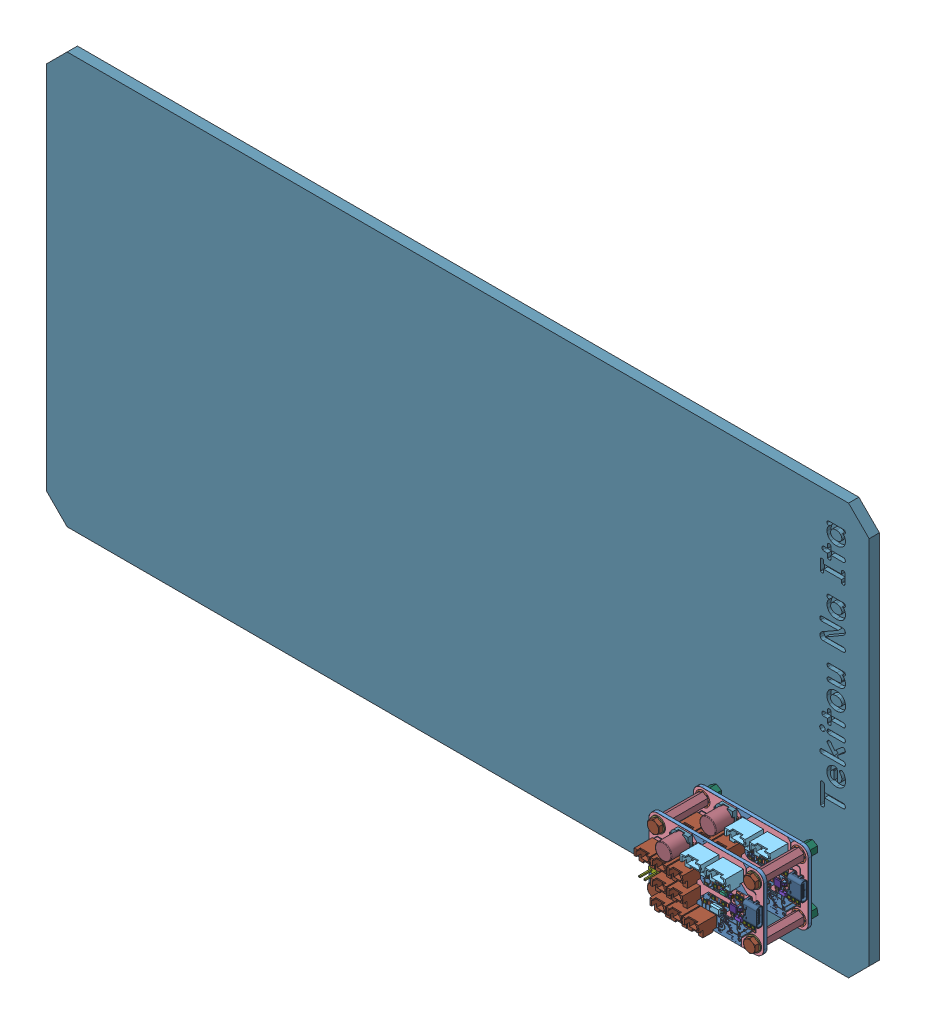
SolidWorks assembly USB_JST-XH_Converter組立サンプル図, configuration ﾃﾞﾌｫﾙﾄ. Lengths in mm. (continued)
Components (placement in the parent): (continued)
- USB_JST-XH_Converter組立図-1: USB_JST-XH_Converter組立図 [ﾃﾞﾌｫﾙﾄ] at (-33.7897 -17.3903 6.5602) size (55.86 35.85 14.61) (continued)
  - Step_Models_f1fe-1: Step_Models_f1fe [ﾃﾞﾌｫﾙﾄ] at origin size (53.92 34.35 13.46) (continued)
    - Top_f1fe_1-1: Top_f1fe_1 [ﾃﾞﾌｫﾙﾄ] at origin size (53.92 34.35 13.46) (continued)
      - R2_RT1220P-101-M004_639B496B-7: R2_RT1220P-101-M004_639B496B [ﾃﾞﾌｫﾙﾄ] at (154.8711 -96.7286 0) x (1 0 0) z (0 -1 0) size (2 0.5 1.25) (continued)
        - RT1220P-101-M002-1: RT1220P-101-M002 [ﾃﾞﾌｫﾙﾄ] at origin size (1.95 0.45 1.25)
        - RT1220P-101-M003-1: RT1220P-101-M003 [ﾃﾞﾌｫﾙﾄ] at origin size (1.2 0.03 1.25)
      - R2_RT1220P-101-M004_639B496B-8: R2_RT1220P-101-M004_639B496B [ﾃﾞﾌｫﾙﾄ] at (156.8711 -101.4286 0) x (1 0 0) z (0 -1 0) size (2 0.5 1.25)
        - RT1220P-101-M-1: RT1220P-101-M [ﾃﾞﾌｫﾙﾄ] at origin size (0.4 0.5 1.25)
        - RT1220P-101-M001-1: RT1220P-101-M001 [ﾃﾞﾌｫﾙﾄ] at origin size (0.4 0.5 1.25)
        - RT1220P-101-M002-1: RT1220P-101-M002 [ﾃﾞﾌｫﾙﾄ] at origin size (1.95 0.45 1.25)
        - RT1220P-101-M003-1: RT1220P-101-M003 [ﾃﾞﾌｫﾙﾄ] at origin size (1.2 0.03 1.25)
      - R2_RT1220P-101-M004_639B496B-9: R2_RT1220P-101-M004_639B496B [ﾃﾞﾌｫﾙﾄ] at (153.2711 -103.4286 0) x (-1 0 0) z (0 1 0) size (2 0.5 1.25)
        - RT1220P-101-M-1: RT1220P-101-M [ﾃﾞﾌｫﾙﾄ] at origin size (0.4 0.5 1.25)
        - RT1220P-101-M001-1: RT1220P-101-M001 [ﾃﾞﾌｫﾙﾄ] at origin size (0.4 0.5 1.25)
        - RT1220P-101-M002-1: RT1220P-101-M002 [ﾃﾞﾌｫﾙﾄ] at origin size (1.95 0.45 1.25)
        - RT1220P-101-M003-1: RT1220P-101-M003 [ﾃﾞﾌｫﾙﾄ] at origin size (1.2 0.03 1.25)
      - R2_RT1220P-101-M004_639B496B-10: R2_RT1220P-101-M004_639B496B [ﾃﾞﾌｫﾙﾄ] at (152.2711 -108.9286 0) x (-1 0 0) z (0 1 0) size (2 0.5 1.25)
        - RT1220P-101-M-1: RT1220P-101-M [ﾃﾞﾌｫﾙﾄ] at origin size (0.4 0.5 1.25)
        - RT1220P-101-M001-1: RT1220P-101-M001 [ﾃﾞﾌｫﾙﾄ] at origin size (0.4 0.5 1.25)
        - RT1220P-101-M002-1: RT1220P-101-M002 [ﾃﾞﾌｫﾙﾄ] at origin size (1.95 0.45 1.25)
        - RT1220P-101-M003-1: RT1220P-101-M003 [ﾃﾞﾌｫﾙﾄ] at origin size (1.2 0.03 1.25)
      - R2_RT1220P-101-M004_639B496B-11: R2_RT1220P-101-M004_639B496B [ﾃﾞﾌｫﾙﾄ] at (157.2711 -108.9286 0) x (-1 0 0) z (0 1 0) size (2 0.5 1.25)
        - RT1220P-101-M-1: RT1220P-101-M [ﾃﾞﾌｫﾙﾄ] at origin size (0.4 0.5 1.25)
        - RT1220P-101-M001-1: RT1220P-101-M001 [ﾃﾞﾌｫﾙﾄ] at origin size (0.4 0.5 1.25)
        - RT1220P-101-M002-1: RT1220P-101-M002 [ﾃﾞﾌｫﾙﾄ] at origin size (1.95 0.45 1.25)
        - RT1220P-101-M003-1: RT1220P-101-M003 [ﾃﾞﾌｫﾙﾄ] at origin size (1.2 0.03 1.25)
      - U2_TLP293(E005_639B4A97-1: U2_TLP293(E005_639B4A97 [ﾃﾞﾌｫﾙﾄ] at (154.5711 -111.9286 0) x (0 -1 0) z (-1 0 0) size (2.6 2.3 7)
        - TLP293(E-1: TLP293(E [ﾃﾞﾌｫﾙﾄ] at origin size (0.38 1.35 1.25)
        - TLP293(E001-1: TLP293(E001 [ﾃﾞﾌｫﾙﾄ] at origin size (0.38 1.35 1.25)
        - TLP293(E002-1: TLP293(E002 [ﾃﾞﾌｫﾙﾄ] at origin size (0.38 1.35 1.25)
        - TLP293(E003-1: TLP293(E003 [ﾃﾞﾌｫﾙﾄ] at origin size (2.6 2.2 4.55)
        - TLP293(E004-1: TLP293(E004 [ﾃﾞﾌｫﾙﾄ] at origin size (0.38 1.35 1.25)
      - R2_RT1220P-101-M004_639B496B-12: R2_RT1220P-101-M004_639B496B [ﾃﾞﾌｫﾙﾄ] at (148.2711 -112.4286 0) x (-1 0 0) z (0 1 0) size (2 0.5 1.25)
        - RT1220P-101-M-1: RT1220P-101-M [ﾃﾞﾌｫﾙﾄ] at origin size (0.4 0.5 1.25)
        - RT1220P-101-M001-1: RT1220P-101-M001 [ﾃﾞﾌｫﾙﾄ] at origin size (0.4 0.5 1.25)
        - RT1220P-101-M002-1: RT1220P-101-M002 [ﾃﾞﾌｫﾙﾄ] at origin size (1.95 0.45 1.25)
        - RT1220P-101-M003-1: RT1220P-101-M003 [ﾃﾞﾌｫﾙﾄ] at origin size (1.2 0.03 1.25)
      - R2_RT1220P-101-M004_639B496B-13: R2_RT1220P-101-M004_639B496B [ﾃﾞﾌｫﾙﾄ] at (169.5711 -111.6286 0) x (0 1 0) z (1 0 0) size (2 0.5 1.25)
        - RT1220P-101-M-1: RT1220P-101-M [ﾃﾞﾌｫﾙﾄ] at origin size (0.4 0.5 1.25)
        - RT1220P-101-M001-1: RT1220P-101-M001 [ﾃﾞﾌｫﾙﾄ] at origin size (0.4 0.5 1.25)
        - RT1220P-101-M002-1: RT1220P-101-M002 [ﾃﾞﾌｫﾙﾄ] at origin size (1.95 0.45 1.25)
        - RT1220P-101-M003-1: RT1220P-101-M003 [ﾃﾞﾌｫﾙﾄ] at origin size (1.2 0.03 1.25)
      - JP1_PinHeader_1x02_P254mm_Vertical_639B4B42-1: JP1_PinHeader_1x02_P254mm_Vertical_639B4B42 [ﾃﾞﾌｫﾙﾄ] at (124.3011 -109.9286 0) x (0 1 0) z (0 0 1) size (2.54 5.08 11.54)
      - TR1_S-Mini-ZKN004_639B4B58-1: TR1_S-Mini-ZKN004_639B4B58 [ﾃﾞﾌｫﾙﾄ] at (164.8711 -111.2286 0) size (2.9 2.5 1.15)
        - S-Mini-ZKN-1: S-Mini-ZKN [ﾃﾞﾌｫﾙﾄ] at origin size (2.9 1.5 1.1)
        - S-Mini-ZKN001-1: S-Mini-ZKN001 [ﾃﾞﾌｫﾙﾄ] at origin size (0.4 0.51 0.85)
        - S-Mini-ZKN002-1: S-Mini-ZKN002 [ﾃﾞﾌｫﾙﾄ] at origin size (0.4 0.51 0.85)
        - S-Mini-ZKN003-1: S-Mini-ZKN003 [ﾃﾞﾌｫﾙﾄ] at origin size (0.4 0.51 0.85)
      - D2_1N914BWT004_639B4B74-1: D2_1N914BWT004_639B4B74 [ﾃﾞﾌｫﾙﾄ] at (167.5711 -106.6286 0) x (0 -1 0) z (-1 0 0) size (1.6 0.7 0.8)
        - 1N914BWT-1: 1N914BWT [ﾃﾞﾌｫﾙﾄ] at origin size (1.2 0.7 0.8)
        - 1N914BWT001-1: 1N914BWT001 [ﾃﾞﾌｫﾙﾄ] at origin size (0.02 0.05 0.5)
        - 1N914BWT002-1: 1N914BWT002 [ﾃﾞﾌｫﾙﾄ] at origin size (0.2 0.2 0.3)
        - 1N914BWT003-1: 1N914BWT003 [ﾃﾞﾌｫﾙﾄ] at origin size (0.2 0.2 0.3)
      - D2_1N914BWT004_639B4B74-2: D2_1N914BWT004_639B4B74 [ﾃﾞﾌｫﾙﾄ] at (160.5711 -101.4286 0) x (1 0 0) z (0 -1 0) size (1.6 0.7 0.8)
        - 1N914BWT-1: 1N914BWT [ﾃﾞﾌｫﾙﾄ] at origin size (1.2 0.7 0.8)
        - 1N914BWT001-1: 1N914BWT001 [ﾃﾞﾌｫﾙﾄ] at origin size (0.02 0.05 0.5)
        - 1N914BWT002-1: 1N914BWT002 [ﾃﾞﾌｫﾙﾄ] at origin size (0.2 0.2 0.3)
        - 1N914BWT003-1: 1N914BWT003 [ﾃﾞﾌｫﾙﾄ] at origin size (0.2 0.2 0.3)
      - D2_1N914BWT004_639B4B74-3: D2_1N914BWT004_639B4B74 [ﾃﾞﾌｫﾙﾄ] at (160.5711 -99.9286 0) x (1 0 0) z (0 -1 0) size (1.6 0.7 0.8)
        - 1N914BWT-1: 1N914BWT [ﾃﾞﾌｫﾙﾄ] at origin size (1.2 0.7 0.8)
        - 1N914BWT001-1: 1N914BWT001 [ﾃﾞﾌｫﾙﾄ] at origin size (0.02 0.05 0.5)
        - 1N914BWT002-1: 1N914BWT002 [ﾃﾞﾌｫﾙﾄ] at origin size (0.2 0.2 0.3)
        - 1N914BWT003-1: 1N914BWT003 [ﾃﾞﾌｫﾙﾄ] at origin size (0.2 0.2 0.3)
      - D2_1N914BWT004_639B4B74-4: D2_1N914BWT004_639B4B74 [ﾃﾞﾌｫﾙﾄ] at (160.5711 -98.4286 0) x (1 0 0) z (0 -1 0) size (1.6 0.7 0.8)
        - 1N914BWT-1: 1N914BWT [ﾃﾞﾌｫﾙﾄ] at origin size (1.2 0.7 0.8)
        - 1N914BWT001-1: 1N914BWT001 [ﾃﾞﾌｫﾙﾄ] at origin size (0.02 0.05 0.5)
        - 1N914BWT002-1: 1N914BWT002 [ﾃﾞﾌｫﾙﾄ] at origin size (0.2 0.2 0.3)
        - 1N914BWT003-1: 1N914BWT003 [ﾃﾞﾌｫﾙﾄ] at origin size (0.2 0.2 0.3)
      - COMP1_part007_639B4BA4-1: COMP1_part007_639B4BA4 [ﾃﾞﾌｫﾙﾄ] at (156.6711 -98.9286 0) x (-1 0 0) z (0 0 1) size (2.39 2.27 1.1)
        - part-1: part [ﾃﾞﾌｫﾙﾄ] at origin size (0.07 0.07 0)
        - part001-1: part001 [ﾃﾞﾌｫﾙﾄ] at origin size (1.35 2.27 1)
        - part002-1: part002 [ﾃﾞﾌｫﾙﾄ] at origin size (0.52 0.41 0.73)
        - part003-1: part003 [ﾃﾞﾌｫﾙﾄ] at origin size (0.52 0.41 0.73)
        - part004-1: part004 [ﾃﾞﾌｫﾙﾄ] at origin size (0.52 0.41 0.73)
        - part005-1: part005 [ﾃﾞﾌｫﾙﾄ] at origin size (0.52 0.41 0.73)
        - part006-1: part006 [ﾃﾞﾌｫﾙﾄ] at origin size (0.52 0.41 0.73)
      - SW2_SMLE1_639B495B-2: SW2_SMLE1_639B495B [ﾃﾞﾌｫﾙﾄ] at (148.5711 -104.8 0) x (-1 0 0) z (0 1 0) size (1.6 0.36 0.8)
      - R2_RT1220P-101-M004_639B496B-14: R2_RT1220P-101-M004_639B496B [ﾃﾞﾌｫﾙﾄ] at (149.3711 -98.9286 0) x (1 0 0) z (0 -1 0) size (2 0.5 1.25)
        - RT1220P-101-M-1: RT1220P-101-M [ﾃﾞﾌｫﾙﾄ] at origin size (0.4 0.5 1.25)
        - RT1220P-101-M001-1: RT1220P-101-M001 [ﾃﾞﾌｫﾙﾄ] at origin size (0.4 0.5 1.25)
        - RT1220P-101-M002-1: RT1220P-101-M002 [ﾃﾞﾌｫﾙﾄ] at origin size (1.95 0.45 1.25)
        - RT1220P-101-M003-1: RT1220P-101-M003 [ﾃﾞﾌｫﾙﾄ] at origin size (1.2 0.03 1.25)
      - POWER_B03B-XASK-1_639B4BD1-1: POWER_B03B-XASK-1_639B4BD1 [ﾃﾞﾌｫﾙﾄ] at (149.5711 -92.9286 0) x (1 0 0) z (0 -1 0) size (10 12.2 6.4)
      - POWER_B03B-XASK-1_639B4BD1-2: POWER_B03B-XASK-1_639B4BD1 [ﾃﾞﾌｫﾙﾄ] at (161.5711 -92.9286 0) x (1 0 0) z (0 -1 0) size (10 12.2 6.4)
      - FET1_ASSEMBLY_639B4C0B-1: FET1_ASSEMBLY_639B4C0B [ﾃﾞﾌｫﾙﾄ] at (157.3711 -104.1286 0) x (0 -1 0) z (0 0 1) size (2.4 2.92 1.2)
        - Body-1: Body [ﾃﾞﾌｫﾙﾄ] at origin size (1.33 2.92 1.15)
        - PinsArrayL002-1: PinsArrayL002 [ﾃﾞﾌｫﾙﾄ] at origin size (0.54 2.39 0.66)
          - PinsArrayL-1: PinsArrayL [ﾃﾞﾌｫﾙﾄ] at origin size (0.54 0.49 0.66)
          - PinsArrayL001-1: PinsArrayL001 [ﾃﾞﾌｫﾙﾄ] at origin size (0.54 0.49 0.66)
        - FilletPinR-1: FilletPinR [ﾃﾞﾌｫﾙﾄ] at origin size (0.54 0.49 0.66)
      - C3_GQM1885C1H8R2CB01J003_639B4C15-1: C3_GQM1885C1H8R2CB01J003_639B4C15 [ﾃﾞﾌｫﾙﾄ] at (161.5711 -110.7786 0) x (-1 0 0) z (0 0 1) size (1.6 0.9 0.8)
        - GQM1885C1H8R2CB01J-1: GQM1885C1H8R2CB01J [ﾃﾞﾌｫﾙﾄ] at origin size (0.35 0.9 0.8)
        - GQM1885C1H8R2CB01J001-1: GQM1885C1H8R2CB01J001 [ﾃﾞﾌｫﾙﾄ] at origin size (0.35 0.9 0.8)
        - GQM1885C1H8R2CB01J002-1: GQM1885C1H8R2CB01J002 [ﾃﾞﾌｫﾙﾄ] at origin size (0.9 0.87 0.77)
      - C4_U2-P_NCH(繝輔ぅ繝ｬ繝・ヨ蠕・004_639B4C24-1: C4_U2-P_NCH(繝輔ぅ繝ｬ繝・ヨ蠕・004_639B4C24 [ﾃﾞﾌｫﾙﾄ] at (137.5711 -91.9286 0) size (8.89 8.31 10.06)
        - U2-P_NCH(繝輔ぅ繝ｬ繝・ヨ蠕・-1: U2-P_NCH(繝輔ぅ繝ｬ繝・ヨ蠕・ [ﾃﾞﾌｫﾙﾄ] at origin size (7.89 7.89 9.01)
        - U2-P_NCH(繝輔ぅ繝ｬ繝・ヨ蠕・001-1: U2-P_NCH(繝輔ぅ繝ｬ繝・ヨ蠕・001 [ﾃﾞﾌｫﾙﾄ] at origin size (8.31 8.31 2)
        - U2-P_NCH(繝輔ぅ繝ｬ繝・ヨ蠕・002-1: U2-P_NCH(繝輔ぅ繝ｬ繝・ヨ蠕・002 [ﾃﾞﾌｫﾙﾄ] at origin size (3.3 0.81 0.25)
        - U2-P_NCH(繝輔ぅ繝ｬ繝・ヨ蠕・003-1: U2-P_NCH(繝輔ぅ繝ｬ繝・ヨ蠕・003 [ﾃﾞﾌｫﾙﾄ] at origin size (3.3 0.81 0.25)
      - U1_WSON10B_Assy_new_ver014_639B4C30-1: U1_WSON10B_Assy_new_ver014_639B4C30 [ﾃﾞﾌｫﾙﾄ] at (162.0711 -108.4286 0) x (0 1 0) z (0 0 1) size (3 3 0.75)
        - WSON10B_Assy_new_ver2-1: WSON10B_Assy_new_ver2 [ﾃﾞﾌｫﾙﾄ] at origin size (3 3 0.7)
        - WSON10B_Assy_new_ver003-1: WSON10B_Assy_new_ver003 [ﾃﾞﾌｫﾙﾄ] at origin size (3 1.65 0.1)
        - WSON10B_Assy_new_ver004-1: WSON10B_Assy_new_ver004 [ﾃﾞﾌｫﾙﾄ] at origin size (0.24 0.4 0.2)
        - WSON10B_Assy_new_ver005-1: WSON10B_Assy_new_ver005 [ﾃﾞﾌｫﾙﾄ] at origin size (0.24 0.4 0.2)
        - WSON10B_Assy_new_ver006-1: WSON10B_Assy_new_ver006 [ﾃﾞﾌｫﾙﾄ] at origin size (0.24 0.4 0.2)
        - WSON10B_Assy_new_ver007-1: WSON10B_Assy_new_ver007 [ﾃﾞﾌｫﾙﾄ] at origin size (0.24 0.4 0.2)
        - WSON10B_Assy_new_ver008-1: WSON10B_Assy_new_ver008 [ﾃﾞﾌｫﾙﾄ] at origin size (0.24 0.4 0.2)
        - WSON10B_Assy_new_ver009-1: WSON10B_Assy_new_ver009 [ﾃﾞﾌｫﾙﾄ] at origin size (0.24 0.4 0.2)
        - WSON10B_Assy_new_ver010-1: WSON10B_Assy_new_ver010 [ﾃﾞﾌｫﾙﾄ] at origin size (0.24 0.4 0.2)
        - WSON10B_Assy_new_ver011-1: WSON10B_Assy_new_ver011 [ﾃﾞﾌｫﾙﾄ] at origin size (0.24 0.4 0.2)
        - WSON10B_Assy_new_ver012-1: WSON10B_Assy_new_ver012 [ﾃﾞﾌｫﾙﾄ] at origin size (0.24 0.4 0.2)
        - WSON10B_Assy_new_ver013-1: WSON10B_Assy_new_ver013 [ﾃﾞﾌｫﾙﾄ] at origin size (0.24 0.4 0.2)
  - M3×10-1: M3×10 [ﾃﾞﾌｫﾙﾄ] at (125.1311 -91.6286 2.52) x (1 0 0) z (0 1 0) size (5.5 7.06 6.35)
  - 平座金-1: 平座金 [ﾃﾞﾌｫﾙﾄ] at (125.1311 -91.6286 0.52) x (1 0 0) z (0 1 0) size (7 0.5 7)
  - M3×10-2: M3×10 [ﾃﾞﾌｫﾙﾄ] at (171.8711 -91.6286 2.52) x (1 0 0) z (0 1 0) size (5.5 7.06 6.35)
  - M3×10-3: M3×10 [ﾃﾞﾌｫﾙﾄ] at (125.1311 -118.3286 2.52) x (1 0 0) z (0 1 0) size (5.5 7.06 6.35)
  - M3×10-4: M3×10 [ﾃﾞﾌｫﾙﾄ] at (171.8711 -118.3286 2.52) x (1 0 0) z (0 1 0) size (5.5 7.06 6.35)
  - 平座金-2: 平座金 [ﾃﾞﾌｫﾙﾄ] at (125.1311 -118.3286 0.52) x (1 0 0) z (0 1 0) size (7 0.5 7)
  - 平座金-3: 平座金 [ﾃﾞﾌｫﾙﾄ] at (171.8711 -118.3286 0.52) x (1 0 0) z (0 1 0) size (7 0.5 7)
  - 平座金-4: 平座金 [ﾃﾞﾌｫﾙﾄ] at (171.8711 -91.6286 0.52) x (1 0 0) z (0 1 0) size (7 0.5 7)
- スペーサ5mm-1: スペーサ5mm [ﾃﾞﾌｫﾙﾄ] at (91.3414 -135.7189 -15.0598) size (5 5.77 40.44)
- スペーサ5mm-2: スペーサ5mm [ﾃﾞﾌｫﾙﾄ] at (138.0814 -109.0189 -15.0598) size (5 5.77 40.44)
- スペーサ5mm-3: スペーサ5mm [ﾃﾞﾌｫﾙﾄ] at (138.0814 -135.7189 -15.0598) x (-0.437332 -0.8993 0) z (0 0 1) size (5 5.77 40.44)
- スペーサ5mm-4: スペーサ5mm [ﾃﾞﾌｫﾙﾄ] at (91.3414 -109.0189 -15.0598) size (5 5.77 40.44)
- 回路固定板-1: 回路固定板 [ﾃﾞﾌｫﾙﾄ] at (165.6286 44.2811 -21.6898) x (0 -1 0) z (0 0 -1) size (200 400 5)
- スペーサ-5: スペーサ [ﾃﾞﾌｫﾙﾄ] at (138.0814 -135.7189 -21.6898) x (0.348297 0.937384 0) z (0 0 1) size (5 5.77 40.44)
- スペーサ-6: スペーサ [ﾃﾞﾌｫﾙﾄ] at (91.3414 -109.0189 -21.6898) size (5 5.77 40.44)
- スペーサ-7: スペーサ [ﾃﾞﾌｫﾙﾄ] at (91.3414 -135.7189 -21.6898) size (5 5.77 40.44)
- スペーサ-8: スペーサ [ﾃﾞﾌｫﾙﾄ] at (138.0814 -109.0189 -21.6798) size (5 5.77 40.44)
- M3×10-1: M3×10 [ﾃﾞﾌｫﾙﾄ] at (138.0814 -135.7189 -28.6898) x (1 0 0) z (0 -1 0) size (5.5 7.06 6.35)
- M3×10-2: M3×10 [ﾃﾞﾌｫﾙﾄ] at (138.0814 -109.0189 -28.6898) x (1 0 0) z (0 -1 0) size (5.5 7.06 6.35)
- M3×10-3: M3×10 [ﾃﾞﾌｫﾙﾄ] at (91.3414 -135.7189 -28.6898) x (1 0 0) z (0 -1 0) size (5.5 7.06 6.35)
- M3×10-4: M3×10 [ﾃﾞﾌｫﾙﾄ] at (91.3414 -109.0189 -28.6898) x (1 0 0) z (0 -1 0) size (5.5 7.06 6.35)
Mates (geometry in assembly coordinates):
- ﾛｯｸ1: lock: unknown of Board_Geoms_f1fe-1; unknown of Step_Models_f1fe-1
- 一致1: coincident aligned: plane of USB_JST-XH_Converter組立図-1/Board_Geoms_f1fe-1/botPads_f1fe-1 through (-33.7897 -17.3903 4.9402) normal (0 0 1); plane of スペーサ-2 through (138.0814 -109.0189 4.9402) normal (0 0 1)
- 同心円1: concentric anti-aligned: circle of USB_JST-XH_Converter組立図-1/M3×10-2; circle of スペーサ-2
- 一致2: coincident aligned: plane of USB_JST-XH_Converter組立図-1/Board_Geoms_f1fe-1/botPads_f1fe-1 through (-33.7897 -17.3903 4.9402) normal (0 0 1); plane of スペーサ-3 through (138.0814 -135.7189 4.9402) normal (0 0 1)
- 同心円2: concentric anti-aligned: circle of USB_JST-XH_Converter組立図-1/M3×10-4; circle of スペーサ-3
- 一致3: coincident aligned: plane of USB_JST-XH_Converter組立図-1/Board_Geoms_f1fe-1/botPads_f1fe-1 through (-33.7897 -17.3903 4.9402) normal (0 0 1); plane of スペーサ-4 through (91.3414 -109.0189 4.9402) normal (0 0 1)
- 同心円3: concentric anti-aligned: circle of USB_JST-XH_Converter組立図-1/M3×10-1; circle of スペーサ-4
- 一致4: coincident aligned: plane of USB_JST-XH_Converter組立図-1/Board_Geoms_f1fe-1/botPads_f1fe-1 through (-33.7897 -17.3903 4.9402) normal (0 0 1); plane of スペーサ-1 through (91.3414 -135.7189 4.9402) normal (0 0 1)
- 同心円4: concentric anti-aligned: circle of USB_JST-XH_Converter組立図-1/M3×10-3; circle of スペーサ-1
- 一致6: coincident anti-aligned: plane of Board_Geoms_f1fe-1/topZones_f1fe-1 through (-33.7897 -17.3903 -15.0598) normal (0 0 1); plane of スペーサ-3 through (138.0814 -135.7189 -15.0598) normal (0 0 -1)
- 同心円5: concentric anti-aligned: cylinder of Board_Geoms_f1fe-1/Pcb_f1fe-1 through (91.3414 -109.0189 -15.0698) axis (0 0 1) radius 1.6; cylinder of スペーサ-4 through (91.3414 -109.0189 4.9402) axis (0 0 -1) radius 1.5
- 同心円6: concentric anti-aligned: cylinder of Board_Geoms_f1fe-1/Pcb_f1fe-1 through (138.0814 -135.7189 -15.0698) axis (0 0 1) radius 1.6; cylinder of スペーサ-3 through (138.0814 -135.7189 4.9402) axis (0 0 -1) radius 1.5
- 一致17: coincident aligned: plane of Board_Geoms_f1fe-1/botPads_f1fe-1 through (-33.7897 -17.3903 -16.6898) normal (0 0 1); plane of スペーサ-6 through (91.3414 -109.0189 -16.6898) normal (0 0 1)
- 同心円17: concentric anti-aligned: cylinder of Board_Geoms_f1fe-1/Pcb_f1fe-1 through (91.3414 -109.0189 -15.0698) axis (0 0 1) radius 1.6; cylinder of スペーサ-6 through (91.3414 -109.0189 -16.6898) axis (0 0 -1) radius 1.5
- 一致18: coincident aligned: plane of Board_Geoms_f1fe-1/botZones_f1fe-1 through (-33.7897 -17.3903 -16.6798) normal (0 0 1); plane of スペーサ-8 through (138.0814 -109.0189 -16.6798) normal (0 0 1)
- 同心円18: concentric anti-aligned: cylinder of Board_Geoms_f1fe-1/Pcb_f1fe-1 through (138.0814 -109.0189 -15.0698) axis (0 0 1) radius 1.6; cylinder of スペーサ-8 through (138.0814 -109.0189 -16.6798) axis (0 0 -1) radius 1.5
- 一致19: coincident aligned: plane of Board_Geoms_f1fe-1/botPads_f1fe-1 through (-33.7897 -17.3903 -16.6898) normal (0 0 1); plane of スペーサ-7 through (91.3414 -135.7189 -16.6898) normal (0 0 1)
- 同心円19: concentric anti-aligned: cylinder of Board_Geoms_f1fe-1/Pcb_f1fe-1 through (91.3414 -135.7189 -15.0698) axis (0 0 1) radius 1.6; cylinder of スペーサ-7 through (91.3414 -135.7189 -16.6898) axis (0 0 -1) radius 1.5
- 一致20: coincident aligned: plane of Board_Geoms_f1fe-1/botPads_f1fe-1 through (-33.7897 -17.3903 -16.6898) normal (0 0 1); plane of スペーサ-5 through (138.0814 -135.7189 -16.6898) normal (0 0 1)
- 同心円20: concentric aligned: cylinder of スペーサ5mm-3 through (138.0814 -135.7189 4.9402) axis (0 0 -1) radius 1.5; cylinder of スペーサ-5 through (138.0814 -135.7189 -16.6898) axis (0 0 -1) radius 1.5
- 一致22: coincident anti-aligned: plane of 回路固定板-1 through (165.6286 44.2811 -21.6898) normal (0 0 1); plane of スペーサ-7 through (91.3414 -135.7189 -21.6898) normal (0 0 -1)
- 同心円24: concentric anti-aligned: cylinder of 回路固定板-1 through (91.3414 -135.7189 -21.6898) axis (0 0 1) radius 1.25; cylinder of スペーサ-7 through (91.3414 -135.7189 -16.6898) axis (0 0 -1) radius 1.5
- 同心円25: concentric anti-aligned: cylinder of 回路固定板-1 through (138.0814 -135.7189 -21.6898) axis (0 0 1) radius 1.25; cylinder of スペーサ-5 through (138.0814 -135.7189 -16.6898) axis (0 0 -1) radius 1.5
- 一致23: coincident anti-aligned: plane of 回路固定板-1 through (165.6286 44.2811 -26.6898) normal (0 0 -1); plane of M3×10-1 through (138.0814 -135.7189 -26.6898) normal (0 0 1)
- 同心円27: concentric anti-aligned: circle of 回路固定板-1; circle of M3×10-1
- 一致27: coincident: plane of 回路固定板-1 through (165.6286 44.2811 -26.6898) normal (0 0 -1); plane of M3×10-2 through (138.0814 -109.0189 -26.6898) normal (0 0 1)
- 同心円28: concentric anti-aligned: circle of 回路固定板-1; circle of M3×10-2
- 一致28: coincident: plane of 回路固定板-1 through (165.6286 44.2811 -26.6898) normal (0 0 -1); plane of M3×10-4 through (91.3414 -109.0189 -26.6898) normal (0 0 1)
- 同心円29: concentric anti-aligned: circle of 回路固定板-1; circle of M3×10-4
- 一致29: coincident: plane of 回路固定板-1 through (165.6286 44.2811 -26.6898) normal (0 0 -1); plane of M3×10-3 through (91.3414 -135.7189 -26.6898) normal (0 0 1)
- 同心円30: concentric anti-aligned: circle of 回路固定板-1; circle of M3×10-3
